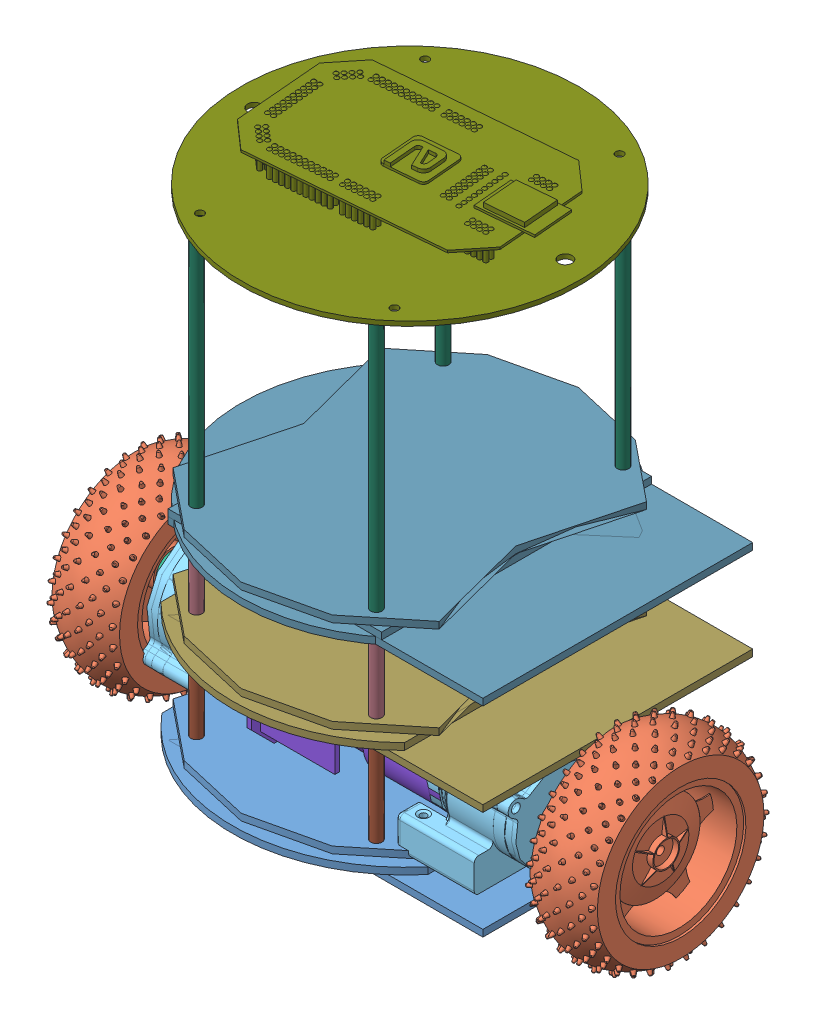
SolidWorks assembly BaseAssembly, configuration Default. Lengths in mm.
Overall size (242.54 275.12 162.15).
36 component instances, 17 part files, 81 mates.
Components (placement in the parent):
- BASE PLATE COMPACT-1: BASE PLATE COMPACT [Default] at (9.1956 73.2306 176.3525) size (151.66 9 157.59)
- 85mm_Wheel-1: 85mm_Wheel [Default] at (-49.5434 86.804 117.1986) x (0 0.469219 0.883082) z (0 -0.883082 0.469219) size (89.76 30.03 89.76)
- Bearing_large-1: Bearing_large [Default] at (149.0346 86.804 117.1064) x (0 0.302035 0.953297) z (-1 0 0) size (34 34 10)
- Bearing_Modifiable-1: Bearing_Modifiable [Default] at (-9.2134 86.804 117.1986) x (0 0 -1) z (1 0 0) size (16 16 5)
- Gear Box Covering - Modifiable-1: Gear Box Covering - Modifiable [Default] at (122.6046 86.804 117.1064) x (0 -0.541121 -0.840945) z (1 0 0) size (87.3 57.46 46.55)
- Gear_Driven - LARGE-1: Gear_Driven - LARGE [Default] at (132.5346 86.804 117.1064) x (0 -0.920513 -0.390712) z (1 0 0) size (41.92 41.92 47.93)
- Gear_Driver-1: Gear_Driver [Default] at (129.4046 103.2 142.587) x (0 0.064546 -0.997915) z (1 0 0) size (21.81 21.81 25.3)
- IG32 MOTORS-1: IG32 MOTORS [Default] at (112.6046 103.2 142.587) x (-1 0 0) z (0 0 1) size (97 41 41.5)
- LINE SENSOR-1: LINE SENSOR [Default] at (106.6956 76.2306 130.3525) x (-1 0 0) z (0 0 1) size (100 13.5 28)
- Motor_Main_Shaft-1: Motor_Main_Shaft [Default] at (112.6046 103.2 142.587) x (0 -0.924225 0.381849) z (1 0 0) size (6 6 15)
- Gear Box Covering - Modifiable-2: Gear Box Covering - Modifiable [Default] at (-9.2134 86.804 117.1986) x (0 -0.541121 0.840945) z (-1 0 0) size (87.3 57.46 46.55)
- IG32 MOTORS-2: IG32 MOTORS [Default] at (0.7866 103.2 91.718) size (97 41 41.5)
- Motor_Main_Shaft-2: Motor_Main_Shaft [Default] at (-14.2134 103.2 91.718) x (0 0 -1) z (1 0 0) size (6 6 15)
- Gear_Driver-2: Gear_Driver [Default] at (-16.0134 103.2 91.718) x (0 0.135257 0.99081) z (-1 0 0) size (21.81 21.81 25.3)
- Gear_Driven - LARGE-2: Gear_Driven - LARGE [Default] at (-19.1434 86.804 117.1986) x (0 0.469219 0.883082) z (-1 0 0) size (41.92 41.92 47.93)
- Bearing_Modifiable-2: Bearing_Modifiable [Default] at (139.0346 103.2 142.587) x (0 -0.922949 -0.384923) z (1 0 0) size (16 16 5)
- Bearing_Modifiable-3: Bearing_Modifiable [Default] at (-30.6434 103.2 91.718) x (0 0.129255 -0.991611) z (1 0 0) size (16 16 5)
- Bearing_Modifiable-4: Bearing_Modifiable [Default] at (122.6046 86.804 117.1064) x (0 0.011286 0.999936) z (-1 0 0) size (16 16 5)
- Bearing_large-2: Bearing_large [Default] at (-35.6434 86.804 117.1986) x (0 0 -1) z (1 0 0) size (34 34 10)
- 85mm_Wheel-2: 85mm_Wheel [Default] at (162.9346 86.804 117.1064) x (0 -0.12189 -0.992544) z (0 -0.992544 0.12189) size (89.76 30.03 89.76)
- 4cm_spacers-1: 4cm_spacers [Default] at (96.6956 124.2306 61.5025) x (0.827993 0 0.560738) z (0 -1 0) size (5 5 50)
- 4cm_spacers-2: 4cm_spacers [Default] at (96.6956 124.2306 171.2025) x (0.889434 0 0.457064) z (0 -1 0) size (5 5 50)
- 4cm_spacers-3: 4cm_spacers [Default] at (16.6956 124.2306 171.2025) x (0.138561 0 0.990354) z (0 -1 0) size (5 5 50)
- 4cm_spacers-4: 4cm_spacers [Default] at (16.6956 124.2306 61.5025) x (0.594628 0 -0.804001) z (0 -1 0) size (5 5 50)
- Floor_Plates1-1: Floor_Plates1 [Default] at (9.1956 121.2306 176.3525) size (151.66 9 157.59)
- 3cm_spacers-1: 3cm_spacers [Default] at (96.6956 172.2306 171.2025) x (1 0 0) z (0 -1 0) size (5 5 40)
- 3cm_spacers-2: 3cm_spacers [Default] at (16.6956 172.2306 171.2025) x (1 0 0) z (0 -1 0) size (5 5 40)
- 3cm_spacers-3: 3cm_spacers [Default] at (16.6956 172.2306 61.5025) x (1 0 0) z (0 -1 0) size (5 5 40)
- 3cm_spacers-4: 3cm_spacers [Default] at (96.6956 172.2306 61.5025) x (1 0 0) z (0 -1 0) size (5 5 40)
- Floor_Plates2-1: Floor_Plates2 [Default] at (9.1956 162.2306 176.3525) size (167.5 9 150)
- 6cm_spacers-1: 6cm_spacers [Default] at (96.6956 285.2306 61.5025) x (1 0 0) z (0 -1 0) size (5 5 125)
- 6cm_spacers-2: 6cm_spacers [Default] at (96.6956 285.2306 171.2025) x (1 0 0) z (0 -1 0) size (5 5 125)
- 6cm_spacers-3: 6cm_spacers [Default] at (16.6956 285.2306 171.2025) x (1 0 0) z (0 -1 0) size (5 5 125)
- 6cm_spacers-4: 6cm_spacers [Default] at (16.6956 285.2306 61.5025) x (1 0 0) z (0 -1 0) size (5 5 125)
- eYFi_Mega-1: eYFi_Mega [Default] at (1.1978 297.2306 100.9903) x (0.084559 0 0.996418) z (-0.996418 0 0.084559) size (150 18 150)
- Hex_Cover-1: Hex_Cover [Default] at (56.6956 76.2306 116.3525) x (0.996418 0 -0.084559) z (0.084559 0 0.996418) size (192.07 186 175) (hidden)
Mates (geometry in assembly coordinates):
- BasePlate_&_LineSensor: coincident anti-aligned: plane of BASE PLATE COMPACT-1 through (127.509 76.2306 116.3525) normal (0 -1 0); plane of LINE SENSOR-1 through (106.6956 76.2306 130.3525) normal (0 1 0)
- Potentiometer&BasePlate: parallel anti-aligned: plane of BASE PLATE COMPACT-1 through (29.6956 84.2306 121.8525) normal (-1 0 0); plane of LINE SENSOR-1 through (28.6956 81.2306 120.8525) normal (1 0 0)
- LineSensor&BasePlate: concentric anti-aligned: cylinder of BASE PLATE COMPACT-1 through (9.1956 84.2306 127.8525) axis (0 -1 0) radius 1.711; cylinder of LINE SENSOR-1 through (9.1956 74.2306 127.8525) axis (0 1 0) radius 1.5
- BasePlate&GearBox1: concentric aligned: cylinder of BASE PLATE COMPACT-1 through (4.0366 68.2306 132.1499) axis (0 1 0) radius 1.75; cylinder of Gear Box Covering - Modifiable-2 through (4.0366 67.8227 132.1499) axis (0 1 0) radius 1.75
- Coincident14: coincident anti-aligned: plane of BASE PLATE COMPACT-1 through (127.509 79.2306 116.3525) normal (0 1 0); plane of Gear Box Covering - Modifiable-2 through (-24.2134 79.2306 117.1986) normal (0 -1 0)
- GearBox&BasePlate1: parallel anti-aligned: plane of BASE PLATE COMPACT-1 through (-2.4644 76.2306 70.2538) normal (-1 0 0); plane of Gear Box Covering - Modifiable-2 through (-4.2134 103.2 91.718) normal (1 0 0)
- BasePlate&GearBox2: concentric aligned: cylinder of BASE PLATE COMPACT-1 through (109.3546 68.2306 102.1551) axis (0 1 0) radius 1.75; cylinder of Gear Box Covering - Modifiable-1 through (109.3546 67.8227 102.1551) axis (0 1 0) radius 1.75
- GearBox&BasePlate2: parallel anti-aligned: plane of BASE PLATE COMPACT-1 through (115.8556 76.2306 70.2538) normal (1 0 0); plane of Gear Box Covering - Modifiable-1 through (117.6046 103.2 142.587) normal (-1 0 0)
- BasePlate&GearBox2C: coincident anti-aligned: plane of BASE PLATE COMPACT-1 through (127.509 79.2306 116.3525) normal (0 1 0); plane of Gear Box Covering - Modifiable-1 through (137.6046 79.2306 117.1064) normal (0 -1 0)
- MotorShaft&GearBox2: concentric aligned: cylinder of IG32 MOTORS-1 through (115.6046 103.2 142.587) axis (-1 0 0) radius 7.5; cylinder of Motor_Main_Shaft-1 through (127.6046 103.2 142.587) axis (-1 0 0) radius 3
- Motor&MotorShaft2: coincident anti-aligned: plane of IG32 MOTORS-1 through (112.6046 103.2 142.587) normal (1 0 0); plane of Motor_Main_Shaft-1 through (112.6046 103.2 142.587) normal (-1 0 0)
- Motor&MotorShaft1: concentric anti-aligned: cylinder of IG32 MOTORS-2 through (-2.2134 103.2 91.718) axis (1 0 0) radius 7.5; cylinder of Motor_Main_Shaft-2 through (0.7866 103.2 91.718) axis (-1 0 0) radius 3
- Motor&MotorShaft11: coincident anti-aligned: plane of IG32 MOTORS-2 through (0.7866 103.2 91.718) normal (-1 0 0); plane of Motor_Main_Shaft-2 through (0.7866 103.2 91.718) normal (1 0 0)
- Motor&GearBox1: concentric aligned: cylinder of Gear Box Covering - Modifiable-2 through (-14.2134 103.2 91.718) axis (1 0 0) radius 10.75; cylinder of IG32 MOTORS-2 through (-2.2134 103.2 91.718) axis (1 0 0) radius 10.5
- Motor&GearBox2: concentric aligned: cylinder of Gear Box Covering - Modifiable-1 through (127.6046 103.2 142.587) axis (-1 0 0) radius 10.75; cylinder of IG32 MOTORS-1 through (115.6046 103.2 142.587) axis (-1 0 0) radius 10.5
- MotorHole&GearBox2: concentric aligned: cylinder of Gear Box Covering - Modifiable-1 through (117.6046 116.7 142.587) axis (1 0 0) radius 1.75; cylinder of IG32 MOTORS-1 through (109.6046 116.7 142.587) axis (1 0 0) radius 1.5
- MotorHole&GearBox1: concentric aligned: cylinder of Gear Box Covering - Modifiable-2 through (-4.2134 116.7 91.718) axis (-1 0 0) radius 1.75; cylinder of IG32 MOTORS-2 through (3.7866 116.7 91.718) axis (-1 0 0) radius 1.5
- Motor2&GearBox2: coincident anti-aligned: plane of Gear Box Covering - Modifiable-2 through (0.7866 103.2 91.718) normal (1 0 0); plane of IG32 MOTORS-2 through (0.7866 103.2 91.718) normal (-1 0 0)
- Motor1&GearBox1: coincident anti-aligned: plane of Gear Box Covering - Modifiable-1 through (112.6046 103.2 142.587) normal (-1 0 0); plane of IG32 MOTORS-1 through (112.6046 103.2 142.587) normal (1 0 0)
- Concentric17: concentric aligned: cylinder of Motor_Main_Shaft-2 through (0.7866 103.2 91.718) axis (-1 0 0) radius 3; cone of Gear_Driver-2 through (-4.2114 103.2 91.718) axis (-1 0 0)
- Coincident25: coincident anti-aligned: plane of Motor_Main_Shaft-2 through (-14.2134 103.2 91.718) normal (-1 0 0); plane of Gear_Driver-2 through (-14.2134 103.2 91.718) normal (1 0 0)
- Concentric18: concentric anti-aligned: cylinder of Gear_Driver-2 through (-16.5134 103.2 91.718) axis (-1 0 0) radius 2.8; cylinder of Bearing_Modifiable-3 through (-30.6434 103.2 91.718) axis (1 0 0) radius 8
- Coincident26: coincident aligned: plane of Gear Box Covering - Modifiable-2 through (-30.6434 109.5417 71.6985) normal (-1 0 0); plane of Bearing_Modifiable-3 through (-30.6434 103.2 91.718) normal (-1 0 0)
- Concentric20: concentric anti-aligned: cylinder of Gear_Driver-1 through (115.4046 103.2 142.587) axis (1 0 0) radius 5.75; cylinder of Motor_Main_Shaft-1 through (127.6046 103.2 142.587) axis (-1 0 0) radius 3
- Coincident27: coincident anti-aligned: plane of Gear_Driver-1 through (127.6046 103.2 142.587) normal (-1 0 0); plane of Motor_Main_Shaft-1 through (127.6046 103.2 142.587) normal (1 0 0)
- Concentric22: concentric aligned: cylinder of Gear_Driver-1 through (129.9046 103.2 142.587) axis (1 0 0) radius 2.8; cylinder of Bearing_Modifiable-2 through (139.0346 103.2 142.587) axis (1 0 0) radius 8
- Coincident28: coincident aligned: plane of Gear Box Covering - Modifiable-1 through (144.0346 109.5417 162.6066) normal (1 0 0); plane of Bearing_Modifiable-2 through (144.0346 103.2 142.587) normal (1 0 0)
- Concentric23: concentric anti-aligned: cylinder of Bearing_Modifiable-1 through (-9.2134 86.804 117.1986) axis (1 0 0) radius 8; cylinder of Gear Box Covering - Modifiable-2 through (-4.2134 86.804 117.1986) axis (-1 0 0) radius 8.75
- Coincident29: coincident aligned: plane of Bearing_Modifiable-1 through (-9.2134 86.804 117.1986) normal (-1 0 0); plane of Gear Box Covering - Modifiable-2 through (-9.2134 103.2 91.718) normal (-1 0 0)
- Concentric24: concentric anti-aligned: cylinder of Gear Box Covering - Modifiable-1 through (117.6046 86.804 117.1064) axis (1 0 0) radius 8.75; cylinder of Bearing_Modifiable-4 through (122.6046 86.804 117.1064) axis (-1 0 0) radius 8
- Coincident30: coincident aligned: plane of Gear Box Covering - Modifiable-1 through (122.6046 103.2 142.587) normal (1 0 0); plane of Bearing_Modifiable-4 through (122.6046 86.804 117.1064) normal (1 0 0)
- Concentric25: concentric aligned: cylinder of Bearing_Modifiable-1 through (-4.2134 86.804 117.1986) axis (-1 0 0) radius 3; cylinder of Gear_Driven - LARGE-2 through (-4.2134 86.804 117.1986) axis (-1 0 0) radius 2.8
- Coincident31: coincident anti-aligned: plane of Gear Box Covering - Modifiable-2 through (-4.2134 86.804 117.1986) normal (-1 0 0); plane of Gear_Driven - LARGE-2 through (-4.2134 86.804 117.1986) normal (1 0 0)
- Concentric26: concentric aligned: cylinder of Gear_Driven - LARGE-1 through (117.6046 86.804 117.1064) axis (1 0 0) radius 2.8; cylinder of Bearing_Modifiable-4 through (117.6046 86.804 117.1064) axis (1 0 0) radius 3
- Coincident32: coincident anti-aligned: plane of Gear Box Covering - Modifiable-1 through (117.6046 86.804 117.1064) normal (1 0 0); plane of Gear_Driven - LARGE-1 through (117.6046 86.804 117.1064) normal (-1 0 0)
- Concentric27: concentric anti-aligned: cylinder of Gear_Driven - LARGE-2 through (-47.9434 86.804 117.1986) axis (1 0 0) radius 7.5; cylinder of Bearing_large-2 through (-25.6434 86.804 117.1986) axis (-1 0 0) radius 7.5
- Concentric28: concentric anti-aligned: cylinder of Bearing_large-1 through (139.0346 86.804 117.1064) axis (1 0 0) radius 7.5; cylinder of Gear_Driven - LARGE-1 through (161.3346 86.804 117.1064) axis (-1 0 0) radius 7.5
- Coincident33: coincident aligned: plane of Gear Box Covering - Modifiable-2 through (-35.6434 86.804 117.1986) normal (-1 0 0); plane of Bearing_large-2 through (-35.6434 86.804 117.1986) normal (-1 0 0)
- Coincident34: coincident aligned: plane of Bearing_large-1 through (149.0346 86.804 117.1064) normal (1 0 0); plane of Gear Box Covering - Modifiable-1 through (149.0346 86.804 117.1064) normal (1 0 0)
- Concentric29: concentric anti-aligned: cylinder of 85mm_Wheel-1 through (-47.9434 86.804 117.1986) axis (-1 0 0) radius 8.5; cylinder of Gear_Driven - LARGE-2 through (-47.9434 86.804 117.1986) axis (1 0 0) radius 7.5
- Parallel1: parallel aligned: plane of 85mm_Wheel-1 through (-47.9434 92.6969 120.8833) normal (0 -0.469219 -0.883082); plane of Gear_Driven - LARGE-2 through (-52.1434 87.0485 110.253) normal (0 -0.469219 -0.883082)
- Coincident39: coincident anti-aligned: plane of 85mm_Wheel-1 through (-52.1434 86.804 117.1986) normal (1 0 0); plane of Gear_Driven - LARGE-2 through (-52.1434 86.804 117.1986) normal (-1 0 0)
- Concentric30: concentric anti-aligned: cylinder of Gear_Driven - LARGE-1 through (161.3346 86.804 117.1064) axis (-1 0 0) radius 7.5; cylinder of 85mm_Wheel-2 through (161.3346 86.804 117.1064) axis (1 0 0) radius 8.5
- Coincident41: coincident anti-aligned: plane of Gear_Driven - LARGE-1 through (165.5346 89.5194 110.7088) normal (0 0.798623 -0.601832); plane of 85mm_Wheel-2 through (161.3346 93.7022 116.2593) normal (0 -0.798623 0.601832)
- Coincident42: coincident anti-aligned: plane of Gear_Driven - LARGE-1 through (165.5346 86.804 117.1064) normal (1 0 0); plane of 85mm_Wheel-2 through (165.5346 86.804 117.1064) normal (-1 0 0)
- Concentric31: concentric anti-aligned: cylinder of BASE PLATE COMPACT-1 through (96.6956 86.2306 61.5025) axis (0 -1 0) radius 1.25; cylinder of 4cm_spacers-1 through (96.6956 74.2306 61.5025) axis (0 1 0) radius 1.25
- Coincident43: coincident anti-aligned: plane of BASE PLATE COMPACT-1 through (127.509 79.2306 116.3525) normal (0 1 0); plane of 4cm_spacers-1 through (96.6956 79.2306 61.5025) normal (0 -1 0)
- Concentric32: concentric anti-aligned: cylinder of BASE PLATE COMPACT-1 through (16.6956 86.2306 61.5025) axis (0 -1 0) radius 1.25; cylinder of 4cm_spacers-4 through (16.6956 74.2306 61.5025) axis (0 1 0) radius 1.25
- Concentric33: concentric anti-aligned: cylinder of BASE PLATE COMPACT-1 through (16.6956 86.2306 171.2025) axis (0 -1 0) radius 1.25; cylinder of 4cm_spacers-3 through (16.6956 74.2306 171.2025) axis (0 1 0) radius 1.25
- Concentric34: concentric anti-aligned: cylinder of BASE PLATE COMPACT-1 through (96.6956 86.2306 171.2025) axis (0 -1 0) radius 1.25; cylinder of 4cm_spacers-2 through (96.6956 74.2306 171.2025) axis (0 1 0) radius 1.25
- Coincident44: coincident anti-aligned: plane of BASE PLATE COMPACT-1 through (127.509 79.2306 116.3525) normal (0 1 0); plane of 4cm_spacers-4 through (16.6956 79.2306 61.5025) normal (0 -1 0)
- Coincident45: coincident anti-aligned: plane of BASE PLATE COMPACT-1 through (127.509 79.2306 116.3525) normal (0 1 0); circle of 4cm_spacers-3
- Coincident46: coincident anti-aligned: plane of BASE PLATE COMPACT-1 through (127.509 79.2306 116.3525) normal (0 1 0); plane of 4cm_spacers-2 through (96.6956 79.2306 171.2025) normal (0 -1 0)
- Concentric35: concentric anti-aligned: cylinder of 4cm_spacers-4 through (16.6956 119.2306 61.5025) axis (0 1 0) radius 1.25; cylinder of Floor_Plates1-1 through (16.6956 134.2306 61.5025) axis (0 -1 0) radius 1.25
- Concentric36: concentric anti-aligned: line of 4cm_spacers-2 through (96.6956 119.2306 171.2025) axis (0 1 0); axis of Floor_Plates1-1 through (96.6956 127.2306 171.2025) axis (0 -1 0)
- Coincident47: coincident anti-aligned: plane of 4cm_spacers-1 through (96.6956 124.2306 61.5025) normal (0 1 0); plane of Floor_Plates1-1 through (127.509 124.2306 116.3525) normal (0 -1 0)
- Concentric37: concentric anti-aligned: cylinder of Floor_Plates1-1 through (16.6956 134.2306 171.2025) axis (0 -1 0) radius 1.25; cylinder of 3cm_spacers-2 through (16.6956 122.2306 171.2025) axis (0 1 0) radius 1.25
- Concentric38: concentric anti-aligned: cylinder of Floor_Plates1-1 through (16.6956 134.2306 61.5025) axis (0 -1 0) radius 1.25; cylinder of 3cm_spacers-3 through (16.6956 122.2306 61.5025) axis (0 1 0) radius 1.25
- Concentric39: concentric anti-aligned: cylinder of Floor_Plates1-1 through (96.6956 134.2306 171.2025) axis (0 -1 0) radius 1.25; cylinder of 3cm_spacers-1 through (96.6956 122.2306 171.2025) axis (0 1 0) radius 1.25
- Concentric40: concentric anti-aligned: cylinder of Floor_Plates1-1 through (96.6956 134.2306 61.5025) axis (0 -1 0) radius 1.25; cylinder of 3cm_spacers-4 through (96.6956 122.2306 61.5025) axis (0 1 0) radius 1.25
- Coincident50: coincident anti-aligned: plane of Floor_Plates1-1 through (127.509 127.2306 116.3525) normal (0 1 0); plane of 3cm_spacers-2 through (16.6956 127.2306 171.2025) normal (0 -1 0)
- Coincident52: coincident anti-aligned: plane of Floor_Plates1-1 through (127.509 127.2306 116.3525) normal (0 1 0); plane of 3cm_spacers-1 through (96.6956 127.2306 171.2025) normal (0 -1 0)
- Coincident53: coincident anti-aligned: plane of Floor_Plates1-1 through (127.509 127.2306 116.3525) normal (0 1 0); plane of 3cm_spacers-3 through (16.6956 127.2306 61.5025) normal (0 -1 0)
- Coincident54: coincident anti-aligned: plane of Floor_Plates1-1 through (127.509 127.2306 116.3525) normal (0 1 0); plane of 3cm_spacers-4 through (96.6956 127.2306 61.5025) normal (0 -1 0)
- Concentric41: concentric anti-aligned: cylinder of 3cm_spacers-3 through (16.6956 157.2306 61.5025) axis (0 1 0) radius 1.25; cylinder of Floor_Plates2-1 through (16.6956 175.2306 61.5025) axis (0 -1 0) radius 1.25
- Concentric42: concentric anti-aligned: cylinder of 3cm_spacers-1 through (96.6956 157.2306 171.2025) axis (0 1 0) radius 1.25; cylinder of Floor_Plates2-1 through (96.6956 175.2306 171.2025) axis (0 -1 0) radius 1.25
- Coincident55: coincident anti-aligned: plane of 3cm_spacers-3 through (16.6956 162.2306 61.5025) normal (0 1 0); plane of Floor_Plates2-1 through (56.6956 162.2306 116.3525) normal (0 -1 0)
- Concentric43: concentric anti-aligned: cylinder of Floor_Plates2-1 through (16.6956 175.2306 61.5025) axis (0 -1 0) radius 1.25; cylinder of 6cm_spacers-4 through (16.6956 160.2306 61.5025) axis (0 1 0) radius 1.25
- Concentric44: concentric anti-aligned: cylinder of Floor_Plates2-1 through (16.6956 175.2306 171.2025) axis (0 -1 0) radius 1.25; cylinder of 6cm_spacers-3 through (16.6956 160.2306 171.2025) axis (0 1 0) radius 1.25
- Concentric45: concentric anti-aligned: cylinder of Floor_Plates2-1 through (96.6956 175.2306 171.2025) axis (0 -1 0) radius 1.25; cylinder of 6cm_spacers-2 through (96.6956 160.2306 171.2025) axis (0 1 0) radius 1.25
- Concentric46: concentric anti-aligned: cylinder of Floor_Plates2-1 through (96.6956 175.2306 61.5025) axis (0 -1 0) radius 1.25; cylinder of 6cm_spacers-1 through (96.6956 160.2306 61.5025) axis (0 1 0) radius 1.25
- Coincident56: coincident anti-aligned: plane of Floor_Plates2-1 through (56.6956 165.2306 116.3525) normal (0 1 0); plane of 6cm_spacers-4 through (16.6956 165.2306 61.5025) normal (0 -1 0)
- Coincident58: coincident anti-aligned: plane of Floor_Plates2-1 through (56.6956 165.2306 116.3525) normal (0 1 0); plane of 6cm_spacers-1 through (96.6956 165.2306 61.5025) normal (0 -1 0)
- Coincident59: coincident anti-aligned: plane of Floor_Plates2-1 through (56.6956 165.2306 116.3525) normal (0 1 0); plane of 6cm_spacers-3 through (16.6956 165.2306 171.2025) normal (0 -1 0)
- Coincident60: coincident anti-aligned: plane of Floor_Plates2-1 through (56.6956 165.2306 116.3525) normal (0 1 0); plane of 6cm_spacers-2 through (96.6956 165.2306 171.2025) normal (0 -1 0)
- Parallel3: parallel anti-aligned: plane of 6cm_spacers-2 through (96.6956 285.2306 171.2025) normal (0 1 0); plane of eYFi_Mega-1 through (56.6956 285.2306 116.3525) normal (0 -1 0)
- Concentric51: concentric aligned: cylinder of Floor_Plates2-1 through (56.6956 162.2306 116.3525) axis (0 1 0) radius 75; cylinder of eYFi_Mega-1 through (56.6956 285.2306 116.3525) axis (0 1 0) radius 75
- Coincident62: coincident aligned: circle of 6cm_spacers-4; plane of eYFi_Mega-1 through (56.6956 285.2306 116.3525) normal (0 -1 0)
- Parallel4: parallel aligned: plane of eYFi_Mega-1 through (5.5949 298.2306 152.8041) normal (0.084559 0 0.996418); plane of Hex_Cover-1 through (13.7573 151.2306 207.8109) normal (0.084559 0 0.996418)
- Concentric52: concentric aligned: cylinder of eYFi_Mega-1 through (56.6956 285.2306 116.3525) axis (0 1 0) radius 75; circle of Hex_Cover-1
- Coincident64: coincident: plane of BASE PLATE COMPACT-1 through (127.509 76.2306 116.3525) normal (0 -1 0); plane of Hex_Cover-1 through (56.6956 76.2306 116.3525) normal (0 -1 0)
